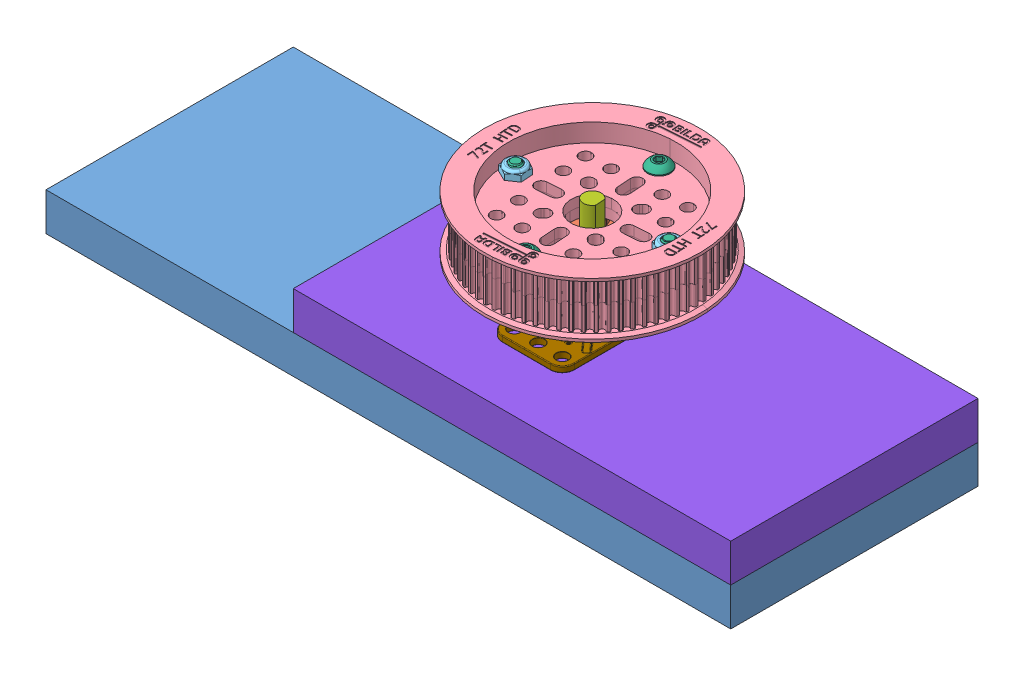
SolidWorks assembly pivotHautElevateur, configuration Défaut. Lengths in mm.
Overall size (228.6 78.41 82.55).
36 component instances, 12 part files, 25 mates.
Components (placement in the parent):
- plaqueHaut-1: plaqueHaut [Défaut] at (326.7894 -14.786 191.3199) x (1 0 0) z (0 -1 0) size (228.6 82.55 12.7)
- 1309-0016-1006 assembly-1: 1309-0016-1006 assembly [Défaut] at (365.0893 27.1876 177.1992) x (0.655754 0 -0.754974) z (0 -1 0) size (28.36 32 10.95)
  - 1309-0016-1006 assembly.STEP-1: 1309-0016-1006 assembly.STEP [Défaut] at origin size (28.36 32 10.95)
    - 1309-0016-1006.STEP-1: 1309-0016-1006.STEP [Défaut] at (-18.2019 0.5776 8.7736) size (25.38 32 10)
    - 2800-0004-0014_90128A207.STEP-1: 2800-0004-0014_90128A207.STEP [Défaut] at (-16.149 11.6963 8.7736) x (0.5 -0.5 -0.707107) z (0.707107 0.707107 0) size (7 7 18.01)
    - 2800-0004-0014_90128A207.STEP-2: 2800-0004-0014_90128A207.STEP [Défaut] at (-20.2547 -10.5411 8.7736) x (-0.5 0.5 -0.707107) z (-0.707107 -0.707107 0) size (7 7 18.01)
- 3402-0014-0072 pulley-1: 3402-0014-0072 pulley [Défaut] at (364.8802 56.6295 250.8953) x (0.070159 0 0.997536) z (0 -1 0) size (71.96 71.96 18.5)
  - 3402-0014-0072 assembly.STEP-1: 3402-0014-0072 assembly.STEP [Défaut] at origin size (71.96 71.96 18.5)
    - 3402-0014-0072.STEP-1: 3402-0014-0072.STEP [Défaut] at (-60.2208 7.0832 38.7155) size (71.96 71.96 10.5)
    - 3402-0014-0072.STEP-2: 3402-0014-0072.STEP [Défaut] at (-60.2208 7.0832 23.2155) x (0 -1 0) z (0 0 -1) size (71.96 71.96 10.5)
    - 2812-0004-0007_90576A103.STEP-1: 2812-0004-0007_90576A103.STEP [Défaut] at (-60.2208 31.0832 29.7155) x (0.866025 0.5 0) z (-0.5 0.866025 0) size (7.02 4.86 8.1)
    - 2812-0004-0007_90576A103.STEP-2: 2812-0004-0007_90576A103.STEP [Défaut] at (-60.2208 -16.9168 29.7155) x (0 1 0) z (-1 0 0) size (7.02 4.86 8.1)
    - 2812-0004-0007_90576A103.STEP-3: 2812-0004-0007_90576A103.STEP [Défaut] at (-84.2208 7.0832 32.2155) x (0.5 0.866025 0) z (0.866025 -0.5 0) size (7.02 4.86 8.1)
    - 2812-0004-0007_90576A103.STEP-4: 2812-0004-0007_90576A103.STEP [Défaut] at (-36.2208 7.0832 32.2155) x (1 0 0) z (0 -1 0) size (7.02 4.86 8.1)
    - 2802-0004-0010_92095A480.STEP-1: 2802-0004-0010_92095A480.STEP [Défaut] at (-36.2208 7.0832 25.5155) x (-0.923728 -0.383049 0) z (0 0 -1) size (13.53 12.99 15.57)
    - 2802-0004-0010_92095A480.STEP-2: 2802-0004-0010_92095A480.STEP [Défaut] at (-84.2208 7.0832 25.5155) x (0.923728 0.383049 0) z (0 0 -1) size (13.53 12.99 15.57)
    - 2802-0004-0010_92095A480.STEP-3: 2802-0004-0010_92095A480.STEP [Défaut] at (-60.2208 31.0832 36.4155) size (13.53 12.99 15.57)
    - 2802-0004-0010_92095A480.STEP-4: 2802-0004-0010_92095A480.STEP [Défaut] at (-60.2208 -16.9168 36.4155) x (-1 0 0) z (0 0 1) size (13.53 12.99 15.57)
- 2101-0006-0300 3 po-1: 2101-0006-0300 3 po [Défaut] at (353.5894 -43.494 191.3199) x (0.070159 0 0.997536) z (-0.997536 0 0.070159) size (6 76.2 5.5)
- blocHautCote-1: blocHautCote [Défaut] at (368.0644 -2.086 191.3199) x (1 0 0) z (0 -1 0) size (146.05 82.55 12.7)
- 1616-0016-0002 plaque-1: 1616-0016-0002 plaque [Défaut] at (353.5894 -27.486 193.3199) size (24 5.02 40)
  - 1616-0016-0002.STEP-1: 1616-0016-0002.STEP [Défaut] at origin size (24 5.02 40)
    - 1616-0016-0002.STEP-1: 1616-0016-0002.STEP [Défaut] at origin size (24 5.02 40)
- 1616-0016-0002 plaque-2: 1616-0016-0002 plaque [Défaut] at (353.5894 -2.086 193.3199) x (-1 0 0) z (0 0 1) size (24 5.02 40)
  - 1616-0016-0002.STEP-1: 1616-0016-0002.STEP [Défaut] at origin size (24 5.02 40)
    - 1616-0016-0002.STEP-1: 1616-0016-0002.STEP [Défaut] at origin size (24 5.02 40)
- 1611-0514-0006 Roulement-1: 1611-0514-0006 Roulement [Défaut] at (353.5894 -32.486 191.3199) x (0.999897 0 0.014368) z (-0.014368 0 0.999897) size (15 5 15)
- 2910-0919-0006 assembly collet-6: 2910-0919-0006 assembly collet [Défaut] at (379.8638 -36.9656 167.7839) x (0.972179 0 -0.234238) z (0.234238 0 0.972179) size (19 9.89 19.83)
  - 2910-0919-0006 assembly.STEP-1: 2910-0919-0006 assembly.STEP [Défaut] at origin size (19 9.89 19.83)
    - 2910-0919-0006.STEP-1: 2910-0919-0006.STEP [Défaut] at (-31.0565 -0.5204 16.7268) size (19 9.5 18.97)
    - 2800-0004-0010_90128A207.STEP-1: 2800-0004-0010_90128A207.STEP [Défaut] at (-24.2865 -0.5204 11.2868) x (0 -0.807243 -0.59022) z (1 0 0) size (7 7 14.01)
- 1611-0514-0006 Roulement-2: 1611-0514-0006 Roulement [Défaut] at (353.5894 2.914 191.3199) x (-0.983829 0 -0.179109) z (-0.179109 0 0.983829) size (15 5 15)
- 2910-0919-0006 assembly collet-7: 2910-0919-0006 assembly collet [Défaut] at (322.5329 7.3936 174.5931) x (-1 0 0) z (0 0 1) size (19 9.89 19.83)
  - 2910-0919-0006 assembly.STEP-1: 2910-0919-0006 assembly.STEP [Défaut] at origin size (19 9.89 19.83)
    - 2910-0919-0006.STEP-1: 2910-0919-0006.STEP [Défaut] at (-31.0565 -0.5204 16.7268) size (19 9.5 18.97)
    - 2800-0004-0010_90128A207.STEP-1: 2800-0004-0010_90128A207.STEP [Défaut] at (-24.2865 -0.5204 11.2868) x (0 -0.807243 -0.59022) z (1 0 0) size (7 7 14.01)
Mates (geometry in assembly coordinates):
- Coaxiale60: concentric: cylinder of 3402-0014-0072 pulley-1/3402-0014-0072 assembly.STEP-1/3402-0014-0072.STEP-2 through (353.5894 29.664 191.3199) axis (0 -1 0) radius 7; cylinder of 2101-0006-0300 3 po-1 through (353.5894 256.506 191.3199) axis (0 -1 0) radius 3
- Parallèle8: parallel: plane of 1309-0016-1006 assembly-1/1309-0016-1006 assembly.STEP-1/1309-0016-1006.STEP-1 through (356.0633 22.6645 191.1459) normal (-0.997536 0 0.070159); plane of 2101-0006-0300 3 po-1 through (356.0832 256.506 191.1445) normal (0.997536 0 -0.070159)
- Coïncidente66: coincident: plane of 1309-0016-1006 assembly-1/1309-0016-1006 assembly.STEP-1/1309-0016-1006.STEP-1 through (353.5894 22.414 191.3199) normal (0 1 0); plane of 3402-0014-0072 pulley-1/3402-0014-0072 assembly.STEP-1/3402-0014-0072.STEP-2 through (353.5894 22.414 191.3199) normal (0 -1 0)
- Coaxiale61: concentric: circle of 1309-0016-1006 assembly-1/1309-0016-1006 assembly.STEP-1/1309-0016-1006.STEP-1; circle of 3402-0014-0072 pulley-1/3402-0014-0072 assembly.STEP-1/3402-0014-0072.STEP-1
- Coaxiale62: concentric: cylinder of blocHautCote-1 through (353.5894 -14.786 191.3199) axis (0 1 0) radius 3.175; cylinder of plaqueHaut-1 through (353.5894 -27.486 191.3199) axis (0 1 0) radius 3.175
- Coïncidente68: coincident: plane of plaqueHaut-1 through (441.0894 -27.486 232.5949) normal (1 0 0); plane of blocHautCote-1 through (441.0894 -14.786 232.5949) normal (1 0 0)
- Coïncidente69: coincident: plane of plaqueHaut-1 through (326.7894 -14.786 191.3199) normal (0 1 0); plane of blocHautCote-1 through (368.0644 -14.786 191.3199) normal (0 -1 0)
- Parallèle9: parallel: plane of plaqueHaut-1 through (441.0894 -27.486 232.5949) normal (1 0 0); plane of 1616-0016-0002 plaque-1/1616-0016-0002.STEP-1/1616-0016-0002.STEP-1 through (365.5894 -32.486 193.3199) normal (1 0 0)
- Coïncidente72: coincident: plane of plaqueHaut-1 through (326.7894 -27.486 191.3199) normal (0 -1 0); plane of 1616-0016-0002 plaque-1/1616-0016-0002.STEP-1/1616-0016-0002.STEP-1 through (353.5894 -27.486 193.3199) normal (0 1 0)
- Coaxiale66: concentric: cylinder of 1616-0016-0002 plaque-1/1616-0016-0002.STEP-1/1616-0016-0002.STEP-1 through (353.5894 -32.486 191.3199) axis (0 1 0) radius 7; cylinder of 1611-0514-0006 Roulement-1 through (353.5894 -32.486 191.3199) axis (0 1 0) radius 3
- Coïncidente73: coincident: plane of 1616-0016-0002 plaque-1/1616-0016-0002.STEP-1/1616-0016-0002.STEP-1 through (353.5894 -28.486 193.3199) normal (0 1 0); plane of 1611-0514-0006 Roulement-1 through (353.5894 -28.486 191.3199) normal (0 -1 0)
- Coaxiale67: concentric: cylinder of 2101-0006-0300 3 po-1 through (353.5894 256.506 191.3199) axis (0 -1 0) radius 3; cylinder of 1611-0514-0006 Roulement-1 through (353.5894 -32.486 191.3199) axis (0 1 0) radius 3
- Coaxiale68: concentric: cylinder of plaqueHaut-1 through (353.5894 -27.486 191.3199) axis (0 1 0) radius 3.175; cylinder of 2101-0006-0300 3 po-1 through (353.5894 256.506 191.3199) axis (0 -1 0) radius 3
- Coaxiale69: concentric: cylinder of 2101-0006-0300 3 po-1 through (353.5894 256.506 191.3199) axis (0 -1 0) radius 3; cylinder of 2910-0919-0006 assembly collet-6/2910-0919-0006 assembly.STEP-1/2910-0919-0006.STEP-1 through (353.5894 -32.986 191.3199) axis (0 -1 0) radius 3
- Coïncidente76: coincident: plane of 1611-0514-0006 Roulement-1 through (353.5894 -32.486 191.3199) normal (0 -1 0); plane of 2910-0919-0006 assembly collet-6/2910-0919-0006 assembly.STEP-1/2910-0919-0006.STEP-1 through (353.5894 -32.486 191.3199) normal (0 1 0)
- Coaxiale70: concentric: cylinder of 2101-0006-0300 3 po-1 through (353.5894 256.506 191.3199) axis (0 -1 0) radius 3; cylinder of 1616-0016-0002 plaque-2/1616-0016-0002.STEP-1/1616-0016-0002.STEP-1 through (353.5894 2.914 191.3199) axis (0 -1 0) radius 7
- Parallèle10: parallel: plane of blocHautCote-1 through (441.0894 -14.786 232.5949) normal (1 0 0); plane of 1616-0016-0002 plaque-2/1616-0016-0002.STEP-1/1616-0016-0002.STEP-1 through (365.5894 2.914 193.3199) normal (1 0 0)
- Coaxiale71: concentric: cylinder of 1616-0016-0002 plaque-2/1616-0016-0002.STEP-1/1616-0016-0002.STEP-1 through (353.5894 2.914 191.3199) axis (0 -1 0) radius 7; cylinder of 1611-0514-0006 Roulement-2 through (353.5894 -1.086 191.3199) axis (0 1 0) radius 7
- Coïncidente78: coincident: plane of 1616-0016-0002 plaque-2/1616-0016-0002.STEP-1/1616-0016-0002.STEP-1 through (353.5894 -1.086 193.3199) normal (0 -1 0); plane of 1611-0514-0006 Roulement-2 through (353.5894 -1.086 191.3199) normal (0 1 0)
- Coïncidente79: coincident: plane of blocHautCote-1 through (368.0644 -2.086 191.3199) normal (0 1 0); plane of 1616-0016-0002 plaque-2/1616-0016-0002.STEP-1/1616-0016-0002.STEP-1 through (353.5894 -2.086 193.3199) normal (0 -1 0)
- Parallèle11: parallel: plane of 1309-0016-1006 assembly-1/1309-0016-1006 assembly.STEP-1/1309-0016-1006.STEP-1 through (356.0633 22.6645 191.1459) normal (-0.997536 0 0.070159); plane of 2101-0006-0300 3 po-1 through (356.0832 256.506 191.1445) normal (0.997536 0 -0.070159)
- Coaxiale72: concentric: cylinder of 1309-0016-1006 assembly-1/1309-0016-1006 assembly.STEP-1/1309-0016-1006.STEP-1 through (353.5894 22.6645 191.3199) axis (0 -1 0) radius 3; cylinder of 2101-0006-0300 3 po-1 through (353.5894 256.506 191.3199) axis (0 -1 0) radius 3
- Coaxiale73: concentric: cylinder of 2101-0006-0300 3 po-1 through (353.5894 256.506 191.3199) axis (0 -1 0) radius 3; cylinder of 2910-0919-0006 assembly collet-7/2910-0919-0006 assembly.STEP-1/2910-0919-0006.STEP-1 through (353.5894 3.414 191.3199) axis (0 1 0) radius 3
- Coïncidente81: coincident: plane of 1611-0514-0006 Roulement-2 through (353.5894 2.914 191.3199) normal (0 1 0); plane of 2910-0919-0006 assembly collet-7/2910-0919-0006 assembly.STEP-1/2910-0919-0006.STEP-1 through (353.5894 2.914 191.3199) normal (0 -1 0)
- Coïncidente83: coincident: plane of 1309-0016-1006 assembly-1/1309-0016-1006 assembly.STEP-1/1309-0016-1006.STEP-1 through (353.5894 12.414 191.3199) normal (0 -1 0); plane of 2910-0919-0006 assembly collet-7/2910-0919-0006 assembly.STEP-1/2910-0919-0006.STEP-1 through (353.5894 12.414 191.3199) normal (0 1 0)
